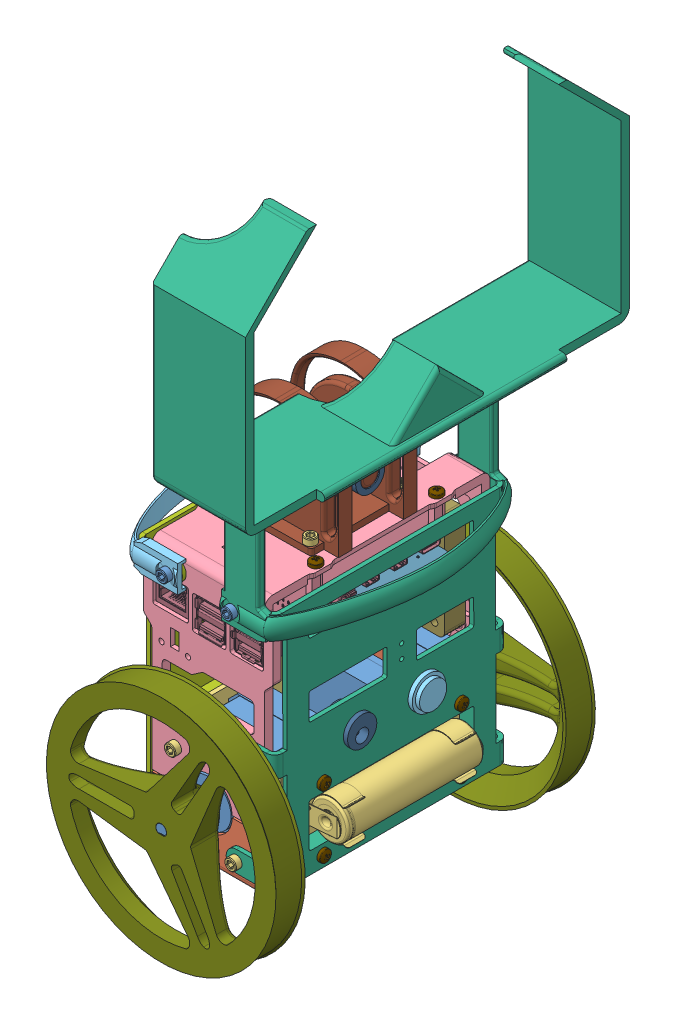
SolidWorks assembly irys5_sc_colector, configuration Domyślna. Lengths in mm.
Overall size (156.29 326.13 184).
91 component instances, 38 part files, 139 mates.
Components (placement in the parent):
- steppermotor-1: steppermotor [Default] at (-42.2578 -7.1789 72.25) size (42.3 42.3 64.5)
- bottomframe_rys3-1: bottomframe_rys3 [Domyślna] at (-43.1924 -29.5373 18.7182) x (0 0 -1) z (0 -1 0) size (108 54 25.86)
- steppermotor-2: steppermotor [Default] at (-42.2578 -7.1789 -31.75) x (-1 0 0) z (0 0 -1) size (42.3 42.3 64.5)
- battery_module-1: battery_module [Domyślna] at (-62.2578 -31.5373 65.25) x (0 0 -1) z (0 -1 0) size (90 40 22.7)
- topframe-1: topframe [Domyślna] at (-44.2495 88.6087 10.8694) x (0 0 -1) z (0 1 0) size (108 62 97.29)
- bumper_front-4: bumper_front [Domyślna] at (-73.7578 82.3211 20.318) x (0 0 -1) z (0 1 0) size (119.34 67.65 21.51)
- bumper_front_colector-3: bumper_front_colector [Domyślna] at (-10.7578 82.314 20.2704) x (0 0 -1) z (0 -1 0) size (184 68.19 188.14)
- imu-1: imu [Domyślna] at (-53.5985 -10.4799 25.3181) x (-0.019519 0 -0.999809) z (0 -1 0) size (10.16 22.86 2.23)
- camera_mounted-1: camera_mounted [Domyślna] at (-50.0059 110.2904 17.0046) x (-0.008727 0 -0.999962) z (0.999897 0.011413 -0.008726) size (25 24 29.88)
  - Camera Module Assem-1: Camera Module Assem [Default] at (-12.4357 -13.5775 -13.0743) size (25 24 24.98)
    - PCB 1-1: PCB 1 [Default] at (8.9736 12.851 19.5114) size (25 24 2.1)
    - Camera Block-1: Camera Block [Default] at (8.9736 15.851 20.5114) size (22 13.5 12.5)
    - Camera end-1: Camera end [Default] at (8.9736 15.851 27.3922) x (0.999924 0.012337 0) z (0 0 1) size (14 14 17.26)
    - Lenz-1: Lenz [Default] at (8.9736 15.851 43.8922) size (9 9 0.5)
    - 15 Pin Ribbon Block Assem-1: 15 Pin Ribbon Block Assem [Default] at (0.7567 20.5462 10.9417) x (1 0 0) z (0 -1 0) size (22 2.5 7)
      - 15 Pin Ribbon Block-1: 15 Pin Ribbon Block [Default] at (8.217 10.8197 14.6952) size (20 2.5 6)
      - Ribbon Clamp-1: Ribbon Clamp [Default] at (8.217 10.8197 14.6952) size (22 2.5 5)
    - 0603 Resistor-1: 0603 Resistor [Default] at (2.3268 23.572 20.4882) size (1.75 0.89 0.66)
    - 0603 Resistor-2: 0603 Resistor [Default] at (4.5768 23.572 20.4882) size (1.75 0.89 0.66)
    - 0603 Resistor-3: 0603 Resistor [Default] at (15.6203 23.5707 20.4857) size (1.75 0.89 0.66)
    - 0603 Resistor-4: 0603 Resistor [Default] at (13.3703 23.5707 20.4857) size (1.75 0.89 0.66)
  - mount-1: mount [Domyślna] at (-15.8432 -12.9016 1.4371) size (25 24 5)
- H-H_M3x12mm-1: H-H_M3x12mm [Predeterminado] at (-51.2078 -23.4959 17.65) x (0.837169 0 0.546944) z (0.546944 0 -0.837169) size (5.77 12 5)
- H-H_M3x6mm-1: H-H_M3x6mm [Predeterminado] at (-51.2078 -14.4959 17.65) x (0.837169 0 0.546944) z (0.546944 0 -0.837169) size (5.77 6 5)
- pan cross head_am-2: pan cross head_am [B18.6.7M - M3 x 0.5 x 6 Type I Cross Recessed PHMS --6N] at (-51.2078 -8.0799 17.65) x (0 -1 0) z (0 0 1) size (8.37 5.6 5.6)
- battery_module_H-2: battery_module_H [Domyślna] at (13.655 -6.0808 19.8906) x (0 0 1) z (-1 0 0) size (90 40 22.7)
  - battery_module-1: battery_module [Domyślna] at (-44.6406 -21.0981 81.7004) size (90 40 22.7)
- pan cross head_am-3: pan cross head_am [B18.6.7M - M3 x 0.5 x 6 Type I Cross Recessed PHMS --6N] at (-78.4454 -22.1789 53.25) size (8.37 5.6 5.6)
- pan cross head_am-4: pan cross head_am [B18.6.7M - M3 x 0.5 x 6 Type I Cross Recessed PHMS --6N] at (-78.4454 7.8211 53.25) size (8.37 5.6 5.6)
- pan cross head_am-5: pan cross head_am [B18.6.7M - M3 x 0.5 x 6 Type I Cross Recessed PHMS --6N] at (-78.4454 7.8211 -12.75) size (8.37 5.6 5.6)
- pan cross head_am-6: pan cross head_am [B18.6.7M - M3 x 0.5 x 6 Type I Cross Recessed PHMS --6N] at (-78.4454 -22.1789 -12.75) size (8.37 5.6 5.6)
- pan cross head_am-7: pan cross head_am [B18.6.7M - M3 x 0.5 x 6 Type I Cross Recessed PHMS --6N] at (-57.2578 -35.9373 53.25) x (0 1 0) z (0 0 1) size (8.37 5.6 5.6)
- pan cross head_am-8: pan cross head_am [B18.6.7M - M3 x 0.5 x 6 Type I Cross Recessed PHMS --6N] at (-27.2578 -35.9373 53.25) x (0 1 0) z (0 0 1) size (8.37 5.6 5.6)
- pan cross head_am-9: pan cross head_am [B18.6.7M - M3 x 0.5 x 6 Type I Cross Recessed PHMS --6N] at (-57.2578 -35.9373 -12.75) x (0 1 0) z (0 0 1) size (8.37 5.6 5.6)
- pan cross head_am-10: pan cross head_am [B18.6.7M - M3 x 0.5 x 6 Type I Cross Recessed PHMS --6N] at (-27.2578 -35.9373 -12.75) x (0 1 0) z (0 0 1) size (8.37 5.6 5.6)
- battery_module_H-3: battery_module_H [Domyślna] at (-98.1705 -8.277 19.8906) x (0 0 1) z (1 0 0) size (90 40 22.7)
  - battery_module-1: battery_module [Domyślna] at (-44.6406 -21.0981 81.7004) size (90 40 22.7)
- pan cross head_am-11: pan cross head_am [B18.6.7M - M3 x 0.5 x 6 Type I Cross Recessed PHMS --6N] at (-6.0701 -22.1789 53.25) x (-1 0 0) z (0 0.924225 0.381849) size (8.37 5.6 5.6)
- pan cross head_am-12: pan cross head_am [B18.6.7M - M3 x 0.5 x 6 Type I Cross Recessed PHMS --6N] at (-6.0701 7.8211 53.25) x (-1 0 0) z (0 0.924225 0.381849) size (8.37 5.6 5.6)
- pan cross head_am-13: pan cross head_am [B18.6.7M - M3 x 0.5 x 6 Type I Cross Recessed PHMS --6N] at (-6.0701 7.8211 -12.75) x (-1 0 0) z (0 0.924225 0.381849) size (8.37 5.6 5.6)
- pan cross head_am-14: pan cross head_am [B18.6.7M - M3 x 0.5 x 6 Type I Cross Recessed PHMS --6N] at (-6.0701 -22.1789 -12.75) x (-1 0 0) z (0 0.924225 0.381849) size (8.37 5.6 5.6)
- M3x6-1: M3x6 [Default] at (-57.7578 82.3211 -40.75) x (0 0 1) z (0.923728 0.383049 0) size (9 5.5 5.5)
- M3x6-2: M3x6 [Default] at (-25.9129 81.3598 -40.6703) x (0 0 1) z (0.923728 0.383049 0) size (9 5.5 5.5)
- M3x4-1: M3x4 [Default] at (-26.7578 24.3211 -38.75) x (0 0 1) z (0.923728 0.383049 0) size (7 5.5 5.5)
- M3x4-2: M3x4 [Default] at (-57.7578 24.3211 -38.75) x (0 0 1) z (0.923728 0.383049 0) size (7 5.5 5.5)
- M3x8-1: M3x8 [Default] at (-26.7578 8.3211 -36.75) x (0 0 1) z (0.923728 0.383049 0) size (9 5.5 5.5)
- M3x8-2: M3x8 [Default] at (-57.7578 8.3211 -36.75) x (0 0 1) z (0.923728 0.383049 0) size (9 5.5 5.5)
- M3x8-3: M3x8 [Default] at (-26.7578 -22.6789 -38.75) x (0 0 1) z (-0.923728 -0.383049 0) size (9 5.5 5.5)
- M3x8-4: M3x8 [Default] at (-57.7578 -22.6789 -38.75) x (0 0 1) z (0.923728 0.383049 0) size (9 5.5 5.5)
- M3x6-3: M3x6 [Default] at (-57.7578 82.3211 81.318) x (0 0 -1) z (-0.923728 -0.383049 0) size (9 5.5 5.5)
- M3x6-4: M3x6 [Default] at (-26.7578 82.3211 81.25) x (0 0 -1) z (-0.923728 -0.383049 0) size (9 5.5 5.5)
- M3x4-3: M3x4 [Default] at (-57.7578 24.3211 79.25) x (0 0 -1) z (-0.923728 -0.383049 0) size (7 5.5 5.5)
- M3x4-4: M3x4 [Default] at (-26.7578 24.3211 79.25) x (0 0 -1) z (-0.923728 -0.383049 0) size (7 5.5 5.5)
- M3x8-5: M3x8 [Default] at (-57.7578 8.3211 77.25) x (0 0 -1) z (-0.923728 -0.383049 0) size (9 5.5 5.5)
- M3x8-6: M3x8 [Default] at (-26.7578 8.314 77.25) x (0 0 -1) z (-0.923728 -0.383049 0) size (9 5.5 5.5)
- M3x8-7: M3x8 [Default] at (-57.7578 -22.6789 79.25) x (0 0 -1) z (-0.923728 -0.383049 0) size (9 5.5 5.5)
- M3x8-8: M3x8 [Default] at (-26.7578 -22.6789 79.25) x (0 0 -1) z (-0.923728 -0.383049 0) size (9 5.5 5.5)
- H-M_M3x10x6mm-1: H-M_M3x10x6mm [Predeterminado] at (-66.7578 78.6087 47.25) size (5.77 16 5)
- H-M_M3x10x6mm-2: H-M_M3x10x6mm [Predeterminado] at (-18.2481 78.6087 47.3511) size (5.77 16 5)
- H-M_M3x10x6mm-5: H-M_M3x10x6mm [Predeterminado] at (-66.7578 78.6087 -10.7875) size (5.77 16 5)
- H-M_M3x10x6mm-6: H-M_M3x10x6mm [Predeterminado] at (-17.7578 78.6087 -10.75) size (5.77 16 5)
- pan cross head_am-15: pan cross head_am [B18.6.7M - M3 x 0.5 x 6 Type I Cross Recessed PHMS --6N] at (-66.7578 93.0087 47.25) x (0 -1 0) z (-0.546944 0 0.837169) size (8.37 5.6 5.6)
- pan cross head_am-16: pan cross head_am [B18.6.7M - M3 x 0.5 x 6 Type I Cross Recessed PHMS --6N] at (-17.7578 93.0087 -10.75) x (0 -1 0) z (-0.546944 0 0.837169) size (8.37 5.6 5.6)
- pan cross head_am-17: pan cross head_am [B18.6.7M - M3 x 0.5 x 6 Type I Cross Recessed PHMS --6N] at (-66.7578 93.0087 -10.75) x (0 -1 0) z (-0.546944 0 0.837169) size (8.37 5.6 5.6)
- pan cross head_am-18: pan cross head_am [B18.6.7M - M3 x 0.5 x 6 Type I Cross Recessed PHMS --6N] at (-17.7578 93.0087 47.25) x (0 -1 0) z (-0.546944 0 0.837169) size (8.37 5.6 5.6)
- switch_simple-1: switch_simple [Domyślna] at (-4.4625 21.3716 4.25) x (0 0 1) z (-0.999997 -0.002583 0) size (16 16 16)
- front-4: front [Domyślna] at (-10.5869 69.5154 20.4189) x (0 0 -1) z (0.002583 -0.999997 0) size (112 23.29 115)
- back-1: back [Domyślna] at (-74.0454 69.4652 19.8764) x (0 0 1) z (0 -1 0) size (112 23.29 115)
- 430250200.stp-4: 430250200.stp [Domyślna] at (-25.0029 52.3587 -6.87) x (-1 0 0) z (0 0 -1) size (5.28 14 10.85)
- 430250200.stp-5: 430250200.stp [Domyślna] at (-40.3546 52.3587 -6.985) x (-1 0 0) z (0 0 -1) size (5.28 14 10.85)
- 430250200.stp-6: 430250200.stp [Domyślna] at (-47.7558 52.3587 -6.985) x (-1 0 0) z (0 0 -1) size (5.28 14 10.85)
- 430250200.stp-7: 430250200.stp [Domyślna] at (-31.8443 52.3587 -6.985) x (-1 0 0) z (0 0 -1) size (5.28 14 10.85)
- M2 x 0.4mm Thread 10mm LONG SOCKET HEAD CAP SCREW-5: M2 x 0.4mm Thread 10mm LONG SOCKET HEAD CAP SCREW [Domyślna] at (-46.1456 112.6087 11.197) x (-0.266178 0.963921 0.002323) z (0.008727 0 0.999962) size (3.8 3.8 12.09)
- M2 x 0.4mm Thread 10mm LONG SOCKET HEAD CAP SCREW-6: M2 x 0.4mm Thread 10mm LONG SOCKET HEAD CAP SCREW [Domyślna] at (-45.9885 112.6087 29.1949) x (-0.999897 -0.011413 0.008726) z (-0.008727 0 -0.999962) size (3.8 3.8 12.09)
- M3x8-9: M3x8 [Default] at (-25.2578 96.6087 -1.75) x (0 -1 0) z (-0.923728 0 0.383049) size (9 5.5 5.5)
- M3x8-13: M3x8 [Default] at (-59.2578 96.6087 42.25) x (0 -1 0) z (-0.923728 0 0.383049) size (9 5.5 5.5)
- M3x8-14: M3x8 [Default] at (-25.2578 96.6087 42.25) x (0 -1 0) z (-0.923728 0 0.383049) size (9 5.5 5.5)
- M3x8-15: M3x8 [Default] at (-59.2578 96.6087 -1.75) x (0 -1 0) z (-0.923728 0 0.383049) size (9 5.5 5.5)
- Panel_Mount_2mm_Power_Plug_v2.step-1: Panel_Mount_2mm_Power_Plug_v2.step [Domyślna] at (-6.4559 21.3664 36.25) x (0 -0.000012 -1) z (-0.002583 0.999997 -0.000012) size (14 13.69 14)
- mount3-1: mount3 [Domyślna] at (-42.0651 90.6087 20.3975) x (-0.008727 0 -0.999962) z (0.999962 0 -0.008727) size (50 53 54.12)
- fan_simple_50x50-1: fan_simple_50x50 [Domyślna] at (-42.2578 53.8211 -24.0253) x (1 0 0) z (0 -1 0) size (50 10 50)
- Raspberry Pi 4 Model B-2: Raspberry Pi 4 Model B [Default] at (-42.2578 77.8087 28.25) x (0 0 1) z (1 0 0) size (88.99 19.91 58.4)
- rys_board_v4.1-1: rys_board_v4.1 [Domyślna] at (-94.2277 65.9587 -55.6601) x (1 0 0) z (0 -1 0) size (56.3 64 18.7)
- LD06_lidar-1: LD06_lidar [Domyślna] at (-75.5201 35.8179 20.34) x (0 0 -1) z (-0.002583 0.999997 0) size (38.59 33.3 38.59)
- Wheel_3x2_spikes-1: Wheel_3x2_spikes [Domyślna] at (-42.2578 -7.1789 96.75) x (0 0 -1) z (0 1 0) size (20 110 110)
- Wheel_3x2_spikes-2: Wheel_3x2_spikes [Domyślna] at (-42.2578 -7.1789 -56.25) x (0 0 1) z (0 1 0) size (20 110 110)
- Servo_LiDAR_hider-1: Servo_LiDAR_hider [Domyślna] at (-36.9556 74.7378 13.3028) x (0.999997 0.002583 0) z (0.002583 -0.999997 0) size (75.64 41.9 38)
  - Servo_DSM44-1: Servo_DSM44 [Default] at (-1.0294 -16.1528 31.7) size (28.2 27.4 8.5)
  - gear-1: gear [Domyślna] at (-4.9294 9.0487 31.7) x (1 0 0) z (0 1 0) size (12.97 12.88 4)
  - lidar_servo_mount-1: lidar_servo_mount [Domyślna] at (-38.6649 6.7422 39.1152) x (0 -1 0) z (0 0 1) size (38 49 38)
  - servo_holder-1: servo_holder [Domyślna] at (-1.0294 -0.0528 38.45) x (-1 0 0) z (0 0 -1) size (40.5 8 19.5)
Mates (geometry in assembly coordinates):
- Koncentryczne1: concentric aligned: cylinder of steppermotor-1 through (-26.7578 -22.6789 64.75) axis (0 0 1) radius 1.25; cylinder of bottomframe_rys3-1 through (-26.7578 -22.6789 74.25) axis (0 0 1) radius 1.6
- Koncentryczne2: concentric aligned: cylinder of steppermotor-1 through (-57.7578 -22.6789 64.75) axis (0 0 1) radius 1.25; cylinder of bottomframe_rys3-1 through (-57.7578 -22.6789 74.25) axis (0 0 1) radius 1.6
- Wspólnie1: coincident anti-aligned: plane of steppermotor-1 through (-64.2538 -29.1749 72.25) normal (0 0 1); plane of bottomframe_rys3-1 through (-42.2578 -7.6789 72.25) normal (0 0 -1)
- Koncentryczne3: concentric aligned: cylinder of bottomframe_rys3-1 through (-57.7578 -22.6789 -33.75) axis (0 0 -1) radius 1.6; cylinder of steppermotor-2 through (-57.7578 -22.6789 -24.25) axis (0 0 -1) radius 1.25
- Koncentryczne4: concentric aligned: circle of bottomframe_rys3-1; cylinder of steppermotor-2 through (-26.7578 -22.6789 -24.25) axis (0 0 -1) radius 1.25
- Wspólnie2: coincident anti-aligned: plane of bottomframe_rys3-1 through (-42.2578 -161.6789 -31.75) normal (0 0 1); plane of steppermotor-2 through (-20.2618 -29.1749 -31.75) normal (0 0 -1)
- Koncentryczne7: concentric aligned: cylinder of steppermotor-2 through (-26.7578 8.3211 -24.25) axis (0 0 -1) radius 1.25; cylinder of topframe-1 through (-26.7578 8.3211 -33.75) axis (0 0 -1) radius 1.6
- Koncentryczne8: concentric aligned: cylinder of steppermotor-1 through (-57.7578 8.3211 64.75) axis (0 0 1) radius 1.25; cylinder of topframe-1 through (-57.7578 8.3211 74.25) axis (0 0 1) radius 1.6
- Wspólnie4: coincident anti-aligned: plane of steppermotor-1 through (-64.2538 -29.1749 72.25) normal (0 0 1); plane of topframe-1 through (-71.2578 51.9927 72.25) normal (0 0 -1)
- Koncentryczne18: concentric aligned: cylinder of bottomframe_rys3-1 through (-26.7578 -22.6789 -33.75) axis (0 0 -1) radius 1.6; cylinder of steppermotor-2 through (-26.7578 -22.6789 -24.25) axis (0 0 -1) radius 1.25
- Koncentryczne55: concentric aligned: cylinder of battery_module-1 through (-51.2078 -29.4959 17.65) axis (0 1 0) radius 1.1; cylinder of imu-1 through (-51.2078 -11.4959 17.65) axis (0 1 0) radius 1.0922
- Koncentryczne56: concentric anti-aligned: cylinder of bottomframe_rys3-1 through (-27.2578 -33.5373 53.25) axis (0 -1 0) radius 1.4; cylinder of battery_module-1 through (-27.2578 -29.4959 53.25) axis (0 1 0) radius 1.6
- Koncentryczne57: concentric anti-aligned: cylinder of bottomframe_rys3-1 through (-57.2578 -33.5373 -12.75) axis (0 -1 0) radius 1.4; cylinder of battery_module-1 through (-57.2578 -29.4959 -12.75) axis (0 1 0) radius 1.6
- Wspólnie27: coincident anti-aligned: plane of bottomframe_rys3-1 through (-42.2578 -31.5373 97.25) normal (0 1 0); plane of battery_module-1 through (-62.2578 -31.5373 65.25) normal (0 -1 0)
- Wspólnie61: coincident anti-aligned: plane of topframe-1 through (-71.2578 88.6087 109.5784) normal (0 -1 0); plane of ToF_nut-5/m2_x_0_4mm_thread_hex_nut-4 through (-37.3526 88.6087 64.7673) normal (0 1 0)
- Koncentryczne104: concentric aligned: cylinder of topframe-1 through (-39.3956 90.6087 53.9072) axis (0 1 0) radius 1.25; cylinder of m2_x_0_4mm_thread_6mm_long_sock-7 through (-39.3956 92.6087 53.9072) axis (0 1 0) radius 1.9
- Wspólnie65: coincident anti-aligned: plane of topframe-1 through (-71.2578 90.6087 109.5784) normal (0 1 0); plane of m2_x_0_4mm_thread_6mm_long_sock-7 through (-39.3956 90.6087 53.9072) normal (0 -1 0)
- Wspólnie67: coincident anti-aligned: plane of topframe-1 through (-71.2578 51.9927 72.25) normal (0 0 -1); plane of ToF_nut-6/m2_x_0_4mm_thread_hex_nut-4 through (-62.7869 47.2984 72.25) normal (0 0 1)
- Wspólnie68: coincident anti-aligned: plane of topframe-1 through (-71.2578 230.6495 -31.75) normal (0 0 1); plane of ToF_nut-7/m2_x_0_4mm_thread_hex_nut-3 through (-34.075 59.7262 -31.75) normal (0 0 -1)
- Wspólnie78: coincident anti-aligned: plane of topframe-1 through (-71.2578 51.9927 74.25) normal (0 0 1); plane of m2_x_0_4mm_thread_6mm_long_sock-15 through (-64.6078 48.6087 74.25) normal (0 0 -1)
- Wspólnie79: coincident anti-aligned: plane of topframe-1 through (-71.2578 51.9927 74.25) normal (0 0 1); plane of m2_x_0_4mm_thread_6mm_long_sock-16 through (-51.9078 48.6087 74.25) normal (0 0 -1)
- Wspólnie80: coincident anti-aligned: plane of topframe-1 through (-71.2578 230.6495 -33.75) normal (0 0 -1); plane of m2_x_0_4mm_thread_6mm_long_sock-17 through (-48.6078 58.3211 -33.75) normal (0 0 1)
- Koncentryczne125: concentric aligned: cylinder of battery_module-1 through (-51.2078 -29.4959 17.65) axis (0 1 0) radius 1.1; cylinder of H-H_M3x12mm-1 through (-51.2078 -29.4959 17.65) axis (0 1 0) radius 1.5
- Wspólnie82: coincident anti-aligned: plane of battery_module-1 through (-62.2578 -29.4959 65.25) normal (0 1 0); plane of H-H_M3x12mm-1 through (-51.2078 -29.4959 17.65) normal (0 -1 0)
- Wspólnie83: coincident anti-aligned: circle of H-H_M3x12mm-1; cylinder of H-H_M3x6mm-1 through (-51.2078 -17.4959 17.65) axis (0 1 0) radius 1.5
- Wspólnie84: coincident anti-aligned: plane of H-H_M3x12mm-1 through (-51.2078 -17.4959 17.65) normal (0 1 0); plane of H-H_M3x6mm-1 through (-51.2078 -17.4959 17.65) normal (0 -1 0)
- Wspólnie85: coincident anti-aligned: plane of imu-1 through (-53.5985 -11.4959 25.3181) normal (0 -1 0); plane of H-H_M3x6mm-1 through (-51.2078 -11.4959 17.65) normal (0 1 0)
- Koncentryczne1261: concentric aligned: cylinder of imu-1 through (-51.2078 -11.4959 17.65) axis (0 1 0) radius 1.0922; cylinder of pan cross head_am-2 through (-51.2078 17.3201 17.65) axis (0 1 0) radius 2.8
- Wspólnie871: coincident anti-aligned: plane of imu-1 through (-53.5985 -10.4799 25.3181) normal (0 1 0); plane of pan cross head_am-2 through (-49.7078 -10.4799 17.65) normal (0 -1 0)
- Koncentryczne1331: concentric aligned: cylinder of bottomframe_rys3-1 through (-57.2578 -33.5373 53.25) axis (0 -1 0) radius 1.4; cylinder of pan cross head_am-7 through (-57.2578 -61.3373 53.25) axis (0 -1 0) radius 2.8
- Wspólnie931: coincident anti-aligned: plane of bottomframe_rys3-1 through (-42.2578 -33.5373 97.25) normal (0 -1 0); plane of pan cross head_am-7 through (-58.7578 -33.5373 53.25) normal (0 1 0)
- Koncentryczne1341: concentric aligned: cylinder of bottomframe_rys3-1 through (-27.2578 -33.5373 53.25) axis (0 -1 0) radius 1.4; cylinder of pan cross head_am-8 through (-27.2578 -61.3373 53.25) axis (0 -1 0) radius 2.8
- Wspólnie941: coincident anti-aligned: plane of bottomframe_rys3-1 through (-42.2578 -33.5373 97.25) normal (0 -1 0); plane of pan cross head_am-8 through (-28.7578 -33.5373 53.25) normal (0 1 0)
- Koncentryczne1351: concentric aligned: cylinder of bottomframe_rys3-1 through (-57.2578 -33.5373 -12.75) axis (0 -1 0) radius 1.4; cylinder of pan cross head_am-9 through (-57.2578 -61.3373 -12.75) axis (0 -1 0) radius 2.8
- Wspólnie951: coincident anti-aligned: plane of bottomframe_rys3-1 through (-42.2578 -33.5373 97.25) normal (0 -1 0); plane of pan cross head_am-9 through (-58.7578 -33.5373 -12.75) normal (0 1 0)
- Koncentryczne1361: concentric aligned: cylinder of bottomframe_rys3-1 through (-27.2578 -33.5373 -12.75) axis (0 -1 0) radius 1.4; cylinder of pan cross head_am-10 through (-27.2578 -61.3373 -12.75) axis (0 -1 0) radius 2.8
- Wspólnie961: coincident anti-aligned: plane of bottomframe_rys3-1 through (-42.2578 -33.5373 97.25) normal (0 -1 0); plane of pan cross head_am-10 through (-28.7578 -33.5373 -12.75) normal (0 1 0)
- Koncentryczne148: concentric aligned: cylinder of topframe-1 through (-26.7578 8.3211 -33.75) axis (0 0 -1) radius 1.6; cylinder of M3x8-1 through (-26.7578 8.3211 -125.4555) axis (0 0 -1) radius 2.75
- Wspólnie107: coincident anti-aligned: plane of topframe-1 through (-71.2578 230.6495 -33.75) normal (0 0 -1); plane of M3x8-1 through (-26.187 6.9447 -33.75) normal (0 0 1)
- Koncentryczne149: concentric aligned: cylinder of topframe-1 through (-57.7578 8.3211 -33.75) axis (0 0 -1) radius 1.6; cylinder of M3x8-2 through (-57.7578 8.3211 -125.4555) axis (0 0 -1) radius 2.75
- Wspólnie108: coincident anti-aligned: plane of topframe-1 through (-71.2578 230.6495 -33.75) normal (0 0 -1); plane of M3x8-2 through (-57.187 6.9447 -33.75) normal (0 0 1)
- Koncentryczne150: concentric aligned: cylinder of bottomframe_rys3-1 through (-57.7578 -22.6789 -33.75) axis (0 0 -1) radius 1.6; cylinder of M3x8-4 through (-57.7578 -22.6789 -127.4555) axis (0 0 -1) radius 2.75
- Koncentryczne153: concentric aligned: circle of topframe-1; cylinder of M3x6-3 through (-57.7578 82.3211 170.0235) axis (0 0 1) radius 2.75
- Koncentryczne155: concentric aligned: cylinder of topframe-1 through (-57.7578 24.3211 74.25) axis (0 0 1) radius 1.6; cylinder of M3x4-3 through (-57.7578 24.3211 167.9555) axis (0 0 1) radius 2.75
- Koncentryczne158: concentric aligned: cylinder of topframe-1 through (-26.7578 8.314 74.25) axis (0 0 1) radius 1.6; cylinder of M3x8-6 through (-26.7578 8.314 165.9555) axis (0 0 1) radius 2.75
- Koncentryczne159: concentric aligned: cylinder of topframe-1 through (-57.7578 8.3211 74.25) axis (0 0 1) radius 1.6; cylinder of M3x8-5 through (-57.7578 8.3211 165.9555) axis (0 0 1) radius 2.75
- Wspólnie115: coincident anti-aligned: plane of topframe-1 through (-71.2578 51.9927 74.25) normal (0 0 1); plane of M3x8-5 through (-57.187 6.9447 74.25) normal (0 0 -1)
- Wspólnie116: coincident anti-aligned: plane of topframe-1 through (-71.2578 51.9927 74.25) normal (0 0 1); plane of M3x8-6 through (-26.187 6.9376 74.25) normal (0 0 -1)
- Równolegle1: parallel aligned: plane of ToF_nut-7/m2_x_0_4mm_thread_hex_nut-1 through (-34.7531 56.3211 -27.53) normal (0 0 1); plane of m2_x_0_4mm_thread_6mm_long_sock-18 through (-35.9078 58.3211 -33.6076) normal (0 0 1)
- Koncentryczne1462: concentric aligned: circle of topframe-1; circle of m2_x_0_4mm_thread_6mm_long_sock-19
- Koncentryczne1463: concentric anti-aligned: circle of bumper2-1; circle of M3x6-7
- Wspólnie970: coincident anti-aligned: plane of bumper2-1 through (-6.0454 102.864 47.0753) normal (1 0 0); plane of M3x6-7 through (-6.0454 81.4447 41.6793) normal (-1 0 0)
- Koncentryczne1464: concentric anti-aligned: circle of bumper2-2; circle of M3x6-8
- Wspólnie971: coincident anti-aligned: plane of bumper2-2 through (-6.0454 102.864 3.0753) normal (1 0 0); plane of M3x6-8 through (-6.0454 81.4447 -2.3207) normal (-1 0 0)
- Koncentryczne1465: concentric aligned: circle of bumper2-1; circle of M3x6-6
- Koncentryczne1466: concentric aligned: circle of bumper2-2; circle of M3x6-5
- Koncentryczne1483: concentric aligned: circle of H-M_M3x10x6mm-1; circle of rys_PCB_rpi_simple-2
- Wspólnie978: coincident anti-aligned: plane of H-M_M3x10x6mm-1 through (-66.7578 78.6087 47.25) normal (0 -1 0); plane of rys_PCB_rpi_simple-2 through (-42.2266 78.6087 28.4747) normal (0 1 0)
- Koncentryczne1484: concentric aligned: circle of H-M_M3x10x6mm-2; circle of rys_PCB_rpi_simple-2
- Wspólnie979: coincident anti-aligned: plane of H-M_M3x10x6mm-2 through (-18.2481 78.6087 47.3511) normal (0 -1 0); plane of rys_PCB_rpi_simple-2 through (-42.2266 78.6087 28.4747) normal (0 1 0)
- Koncentryczne1485: concentric aligned: circle of H-M_M3x10x6mm-5; circle of rys_PCB_rpi_simple-2
- Wspólnie980: coincident anti-aligned: plane of H-M_M3x10x6mm-5 through (-66.7578 78.6087 -10.7875) normal (0 -1 0); plane of rys_PCB_rpi_simple-2 through (-42.2266 78.6087 28.4747) normal (0 1 0)
- Koncentryczne1486: concentric aligned: circle of H-M_M3x10x6mm-6; circle of rys_PCB_rpi_simple-2
- Wspólnie981: coincident anti-aligned: plane of H-M_M3x10x6mm-6 through (-17.7578 78.6087 -10.75) normal (0 -1 0); plane of rys_PCB_rpi_simple-2 through (-42.2266 78.6087 28.4747) normal (0 1 0)
- Koncentryczne1487: concentric anti-aligned: circle of topframe-1; circle of H-M_M3x10x6mm-1
- Wspólnie982: coincident anti-aligned: plane of topframe-1 through (-71.2578 88.6087 109.5784) normal (0 -1 0); plane of H-M_M3x10x6mm-1 through (-66.7578 88.6087 47.25) normal (0 1 0)
- Koncentryczne1490: concentric aligned: circle of topframe-1; circle of M3X6_PLASTIC-2
- Wspólnie983: coincident aligned: plane of topframe-1 through (-71.2578 90.6087 109.5784) normal (0 1 0); circle of M3X6_PLASTIC-2
- Koncentryczne1491: concentric aligned: circle of topframe-1; circle of M3X6_PLASTIC-3
- Wspólnie985: coincident aligned: plane of topframe-1 through (-71.2578 90.6087 109.5784) normal (0 1 0); circle of M3X6_PLASTIC-3
- Koncentryczne1492: concentric aligned: circle of topframe-1; circle of M3X6_PLASTIC-1
- Wspólnie986: coincident aligned: plane of topframe-1 through (-71.2578 90.6087 109.5784) normal (0 1 0); circle of M3X6_PLASTIC-1
- Koncentryczne1493: concentric aligned: circle of topframe-1; circle of M3X6_PLASTIC-4
- Wspólnie987: coincident aligned: plane of topframe-1 through (-71.2578 90.6087 109.5784) normal (0 1 0); circle of M3X6_PLASTIC-4
- Stycznie1: tangent: circle of topframe-1; circle of front-4
- Koncentryczne1502: concentric aligned: circle of topframe-1; circle of front-4
- Wspólnie1015: coincident anti-aligned: plane of topframe-1 through (-71.2578 90.6087 109.5784) normal (0 1 0); plane of m2_x_0_4mm_thread_6mm_long_sock-19 through (-39.3956 90.6087 66.6072) normal (0 -1 0)
- Równolegle8: parallel anti-aligned: plane of rys_PCB_rpi_simple-2 through (-27.3114 55.3587 -4.0403) normal (0 -1 0); plane of 430250200.stp-4 through (-26.9279 56.0087 -3.44) normal (0 1 0)
- Wspólnie1024: coincident anti-aligned: plane of rys_PCB_rpi_simple-2 through (-50.9865 55.3587 -4.0153) normal (0 -1 0); plane of 430250200.stp-6 through (-49.6808 56.0087 -3.555) normal (0 1 0)
- Wspólnie1025: coincident anti-aligned: plane of rys_PCB_rpi_simple-2 through (-43.1115 55.3587 -4.0153) normal (0 -1 0); plane of 430250200.stp-5 through (-42.2796 56.0087 -3.555) normal (0 1 0)
- Wspólnie1026: coincident anti-aligned: plane of rys_PCB_rpi_simple-2 through (-35.2115 55.3587 -4.0153) normal (0 -1 0); plane of 430250200.stp-7 through (-33.7693 56.0087 -3.555) normal (0 1 0)
- Koncentryczne1524: concentric aligned: circle of mount2-1; circle of M3x8-13
- Wspólnie1031: coincident anti-aligned: plane of mount2-1 through (-60.7578 93.6087 -3.25) normal (0 1 0); plane of M3x8-13 through (-58.687 93.6087 43.6264) normal (0 -1 0)
- Koncentryczne1525: concentric aligned: circle of mount2-1; circle of M3x8-14
- Koncentryczne1526: concentric aligned: circle of mount2-1; circle of M3x8-15
- Koncentryczne1527: concentric aligned: circle of mount2-1; circle of M3x8-9
- Wspólnie1032: coincident aligned: plane of mount2-1 through (-60.7578 93.6087 -3.25) normal (0 1 0); circle of M3x8-14
- Wspólnie1033: coincident aligned: plane of mount2-1 through (-60.7578 93.6087 -3.25) normal (0 1 0); circle of M3x8-15
- Wspólnie1034: coincident anti-aligned: plane of mount2-1 through (-60.7578 93.6087 -3.25) normal (0 1 0); plane of M3x8-9 through (-24.687 93.6087 -0.3736) normal (0 -1 0)
- Koncentryczne1531: concentric anti-aligned: circle of mount2-1; circle of M2 x 0.4mm Thread 10mm LONG SOCKET HEAD CAP SCREW-6
- Wspólnie1036: coincident anti-aligned: plane of mount2-1 through (-42.2578 133.6087 39.25) normal (0 0 1); plane of M2 x 0.4mm Thread 10mm LONG SOCKET HEAD CAP SCREW-6 through (-45.9012 112.6087 39.1945) normal (-0.008727 0 -0.999962)
- Koncentryczne1533: concentric aligned: circle of mount2-1; circle of M2 x 0.4mm Thread 10mm LONG SOCKET HEAD CAP SCREW-5
- Wspólnie1038: coincident anti-aligned: plane of mount2-1 through (-42.2578 133.6087 1.25) normal (0 0 -1); plane of M2 x 0.4mm Thread 10mm LONG SOCKET HEAD CAP SCREW-5 through (-46.2328 112.6087 1.1974) normal (0.008727 0 0.999962)
- Koncentryczne1535: concentric aligned: circle of M3x8-9; circle of mount3-1
- Wspólnie1051: coincident anti-aligned: plane of topframe-1 through (-71.2578 90.6087 109.5784) normal (0 1 0); plane of mount3-1 through (-60.7695 90.6087 -2.9402) normal (0 -1 0)
- Koncentryczne1539: concentric aligned: circle of M2 x 0.4mm Thread 10mm LONG SOCKET HEAD CAP SCREW-6; circle of mount3-1
- Koncentryczne1540: concentric anti-aligned: circle of M2 x 0.4mm Thread 10mm LONG SOCKET HEAD CAP SCREW-5; circle of mount3-1
- Wspólnie1053: coincident aligned: circle of camera_mounted-1/mount-1; circle of mount3-1
- Koncentryczne1541: concentric anti-aligned: circle of topframe-1; circle of m2_x_0_4mm_thread_6mm_long_sock-18
- Koncentryczne1542: concentric anti-aligned: circle of topframe-1; circle of m2_x_0_4mm_thread_6mm_long_sock-17
- Koncentryczne1543: concentric aligned: circle of ToF_nut-7/vl53l1x-1; circle of m2_x_0_4mm_thread_6mm_long_sock-17
- Koncentryczne1544: concentric anti-aligned: circle of topframe-1; circle of fan_simple_50x50-1
- Wspólnie1055: coincident anti-aligned: plane of rys_PCB_rpi_simple-2 through (-14.2266 78.6087 -14.0253) normal (0 0 -1); plane of fan_simple_50x50-1 through (-64.2578 31.8211 -14.0253) normal (0 0 1)
- Koncentryczne1545: concentric aligned: circle of steppermotor-1; circle of Wheel_new-1
- Wspólnie1061: coincident aligned: plane of steppermotor-1 through (-44.8633 -9.2845 96.75) normal (0 0 1); plane of Wheel_new-1 through (-28.7585 -61.3214 96.75) normal (0 0 1)
- Koncentryczne1547: concentric aligned: circle of steppermotor-2; circle of Wheel_new-2
- Wspólnie1062: coincident aligned: plane of steppermotor-2 through (-39.6522 -9.2845 -56.25) normal (0 0 -1); plane of Wheel_new-2 through (-55.757 -61.3214 -56.25) normal (0 0 -1)
- Koncentryczne1548: concentric aligned: circle of topframe-1; circle of ToF_nut-6/m2_x_0_4mm_thread_hex_nut-3
- Koncentryczne1549: concentric aligned: circle of topframe-1; circle of m2_x_0_4mm_thread_6mm_long_sock-15
- Koncentryczne1550: concentric aligned: circle of topframe-1; circle of m2_x_0_4mm_thread_6mm_long_sock-16
- Koncentryczne1554: concentric aligned: circle of topframe-1; circle of bumper_front-3
- Koncentryczne1555: concentric anti-aligned: circle of topframe-1; circle of bumper_front-2
- Koncentryczne1556: concentric anti-aligned: circle of H-M_M3x10x6mm-1; circle of Raspberry Pi 4 Model B-2
- Koncentryczne1559: concentric aligned: circle of topframe-1; circle of pan cross head_am-16
- Koncentryczne1560: concentric aligned: circle of topframe-1; circle of H-M_M3x10x6mm-6
- Koncentryczne1561: concentric aligned: circle of H-M_M3x10x6mm-6; circle of Raspberry Pi 4 Model B-2
- Wspólnie1066: coincident anti-aligned: plane of topframe-1 through (-71.2578 88.6087 109.5784) normal (0 -1 0); plane of H-M_M3x10x6mm-2 through (-18.2481 88.6087 47.3511) normal (0 1 0)
- Wspólnie1067: coincident anti-aligned: plane of H-M_M3x10x6mm-2 through (-18.2481 78.6087 47.3511) normal (0 -1 0); plane of Raspberry Pi 4 Model B-2 through (-42.2578 78.6087 28.25) normal (0 1 0)
- Wspólnie1075: coincident aligned: line of Raspberry Pi 4 Model B-2 through (-68.3478 74.5087 -5.56) axis (0 0 -1); line of rys_board_v4.1-1 through (-68.3478 74.5087 -5.2) axis (0 0 -1)
- Wspólnie1076: coincident aligned: line of Raspberry Pi 4 Model B-2 through (-68.3478 74.5087 -6.2) axis (1 0 0); line of rys_board_v4.1-1 through (-68.3478 74.5087 -6.2) axis (1 0 0)
- Wspólnie1078: coincident aligned: line of 430250200.stp-4 through (-26.2029 56.0087 -4.17) axis (1 0 0); line of rys_board_v4.1-1 through (-24.6976 56.0087 -4.17) axis (1 0 0)
- Wspólnie1079: coincident aligned: line of 430250200.stp-7 through (-30.6443 56.0087 -9.685) axis (-1 0 0); line of rys_board_v4.1-1 through (-30.0576 56.0087 -9.685) axis (-1 0 0)
- Wspólnie1080: coincident aligned: line of 430250200.stp-5 through (-39.1546 56.0087 -6.685) axis (-1 0 0); line of rys_board_v4.1-1 through (-37.9576 56.0087 -6.685) axis (-1 0 0)
- Wspólnie1081: coincident aligned: line of 430250200.stp-6 through (-46.5558 56.0087 -9.685) axis (-1 0 0); line of rys_board_v4.1-1 through (-45.8326 56.0087 -9.685) axis (-1 0 0)
- Zablokuj1: lock: unknown of topframe-1; unknown of back-1
- Wspólnie1085: coincident anti-aligned: line of back-1 through (-74.0454 42.3211 39.3764) axis (0 0 1); line of lidar_holder-1 through (-74.0454 44.5211 44.3764) axis (0 0 -1)
- Wspólnie1086: coincident anti-aligned: line of back-1 through (-74.0454 52.3211 39.3764) axis (0 -1 0); line of lidar_holder-1 through (-74.0454 44.5211 39.3764) axis (0 1 0)
- Koncentryczne1562: concentric anti-aligned: circle of lidar_holder-1; circle of k-push-1
- Wspólnie1089: coincident anti-aligned: plane of lidar_holder-1 through (-58.0454 37.0211 20.0764) normal (-1 0 0); plane of k-push-1 through (-58.0454 37.0211 20.0764) normal (1 0 0)
- Wspólnie1090: coincident anti-aligned: plane of lidar_holder-1 through (-58.0454 37.0211 20.0764) normal (-1 0 0); plane of k-push-2 through (-58.0454 39.0211 32.3764) normal (1 0 0)
- Koncentryczne1566: concentric aligned: circle of lidar_mount-1; circle of k-push-1
- Koncentryczne1567: concentric anti-aligned: circle of steppermotor-1; circle of Wheel_3x2_spikes-1
- Koncentryczne1569: concentric anti-aligned: circle of steppermotor-2; circle of Wheel_3x2_spikes-2
- Wspólnie1097: coincident aligned: plane of steppermotor-2 through (-39.6522 -9.2845 -56.25) normal (0 0 -1); plane of Wheel_3x2_spikes-2 through (11.2422 -7.1789 -56.25) normal (0 0 -1)
- Wspólnie1098: coincident anti-aligned: line of LD06_lidar-1 through (-75.5635 52.6143 1.045) axis (0.002583 -0.999997 0); line of Servo_LiDAR_hider-1/lidar_servo_mount-1 through (-75.4832 21.5229 1.045) axis (-0.002583 0.999997 0)
- Wspólnie1099: coincident aligned: line of LD06_lidar-1 through (-75.4702 16.5229 3.5435) axis (0 0 1); line of Servo_LiDAR_hider-1/lidar_servo_mount-1 through (-75.4702 16.5229 6.045) axis (0 0 1)
- Koncentryczne1570: concentric anti-aligned: circle of front-4; circle of Panel_Mount_2mm_Power_Plug_v2.step-1
- Wspólnie1109: coincident anti-aligned: plane of front-4 through (-8.62 82.361 91.25) normal (0.999997 0.002583 0); plane of Panel_Mount_2mm_Power_Plug_v2.step-1 through (-8.4625 21.3612 36.25) normal (-0.999997 -0.002583 0)
- Koncentryczne1571: concentric aligned: circle of front-4; circle of Servo_LiDAR_hider-1/servo_holder-1
